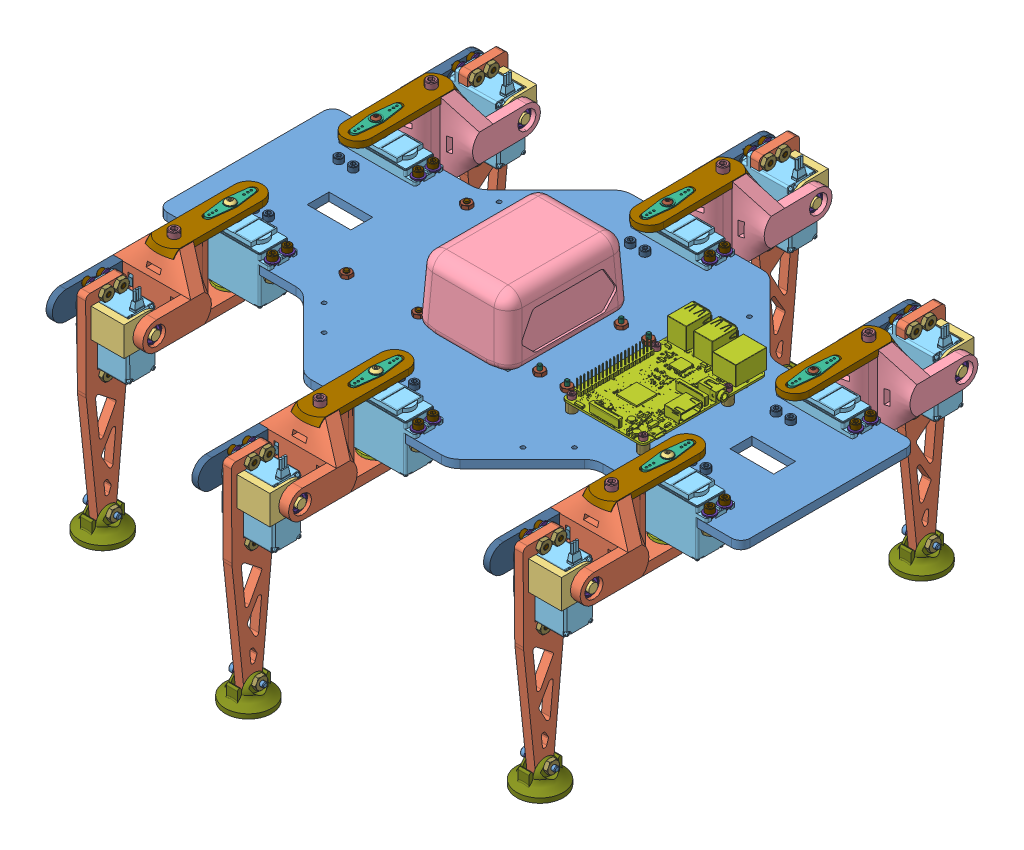
SolidWorks assembly Hexapod, configuration Défaut. Lengths in mm.
Overall size (400 185.52 400.77).
362 component instances, 31 part files, 135 mates.
Components (placement in the parent):
- Body-1: Body [Default] at (-400 -5.6 40) x (1 0 0) z (0 1 0) size (400 220 5.6)
- Leg_(Straight_Foot)-1: Leg_(Straight_Foot) [Default] at (-69.94 -26.67 -0.094) size (71.21 162.26 125.97) (flexible)
  - Foot_(Straight)-1: Foot_(Straight) [Default] at (4.9357 4.6704 -91.3697) x (0.014203 -0.004273 0.99989) z (-0.999899 0 0.014203) size (28 145.4 6)
  - bearing_mount_foot-1: bearing_mount_foot [Default] at (4.8169 16.6442 -99.7278) x (-0.014203 0.004273 -0.99989) z (0.999899 0 -0.014203) size (25 20 29.5)
  - Joint-1: Joint [Défaut] at (35.768 26.4662 -54.7315) x (-0.014203 0 -0.999899) z (0 1 0) size (96.52 53.26 53.26)
  - hs-422-2: hs-422 [Défaut] at (5.1023 6.612 -77.4562) x (-0.014203 0.004273 -0.99989) z (0.000061 0.999991 0.004272) size (19.81 42.09 58.23)
  - hs-422-3: hs-422 [Défaut] at (19.939 20.701 -19.812) x (0 0 1) z (-1 0 0) size (19.81 42.09 58.23)
  - hs-422_horn_straight-1: hs-422_horn_straight [Default] at (-16.9088 16.9412 -87.0065) x (0.014203 0 0.999899) z (0 1 0) size (33.93 4.93 8.79)
  - hs-422_horn_straight-2: hs-422_horn_straight [Default] at (9.652 42.5743 -9.906) x (-0.014203 0 -0.999899) z (-0.999899 0 0.014203) size (33.93 4.93 8.79)
  - Bearing_mount_leg-1: Bearing_mount_leg [Default] at (9.652 21 2.594) x (0 0 1) z (0 -1 0) size (35 20 30)
  - Bearing-1: Bearing [Default] at (9.652 -6.7498 -9.906) x (0.84763 0 0.530588) z (-0.530588 0 0.84763) size (13.87 4.75 13.87)
  - Bearing-2: Bearing [Default] at (32.2403 16.9412 -87.7047) x (0.007588 -0.845349 0.534161) z (-0.012007 -0.534214 -0.845264) size (13.87 4.75 13.87)
  - Joint_attachment_leg-1: Joint_attachment_leg [Défaut] at (35.768 26.4662 -54.7315) x (-0.014203 0 -0.999899) z (0 1 0) size (74.32 19.07 4.32)
  - Joint_attachment_foot-1: Joint_attachment_foot [Défaut] at (35.768 26.4662 -54.7315) x (-0.014203 0 -0.999899) z (0 1 0) size (64.08 6.7 19.07)
  - SBHCSCREW 0.112-40x0.25-HX-N-2: SBHCSCREW 0.112-40x0.25-HX-N [SBHCSCREW 0.112-40x0.25-HX-N] at (-19.9057 16.9412 -86.964) x (0.999899 0 -0.014203) z (-0.007102 0.866025 -0.49995) size (7.85 5.41 5.41)
  - SBHCSCREW 0.112-40x0.25-HX-N-3: SBHCSCREW 0.112-40x0.25-HX-N [SBHCSCREW 0.112-40x0.25-HX-N] at (9.652 45.5715 -9.906) x (0 -1 0) z (0.87304 0 0.487649) size (7.85 5.41 5.41)
  - MSHXNUT 0.138-32-D-N-15: MSHXNUT 0.138-32-D-N [MSHXNUT 0.138-32-D-N] at (5.0634 -17.1179 -82.3793) x (0.012331 0.496295 0.868066) z (-0.999899 0 0.014203) size (7.92 9.15 2.9)
  - MSHXNUT 0.138-32-D-N-16: MSHXNUT 0.138-32-D-N [MSHXNUT 0.138-32-D-N] at (4.9191 -17.0756 -92.5381) x (-0.01227 0.503696 -0.863794) z (-0.999899 0 0.014203) size (7.92 9.15 2.9)
  - MSHXNUT 0.138-32-D-N-17: MSHXNUT 0.138-32-D-N [MSHXNUT 0.138-32-D-N] at (5.0662 30.3817 -82.1827) x (0.000061 0.999991 0.004272) z (-0.999899 0 0.014203) size (7.92 9.15 2.9)
  - MSHXNUT 0.138-32-D-N-18: MSHXNUT 0.138-32-D-N [MSHXNUT 0.138-32-D-N] at (4.9219 30.4239 -92.3416) x (0.000061 0.999991 0.004272) z (-0.999899 0 0.014203) size (7.92 9.15 2.9)
  - HX-SHCS 0.164-32x0.5x0.5-N-1: HX-SHCS 0.164-32x0.5x0.5-N [HX-SHCS 0.164-32x0.5x0.5-N] at (9.1052 47.8568 -48.4) x (0 -1 0) z (0.014203 0 0.999899) size (16.87 6.86 6.86)
  - HX-SHCS 0.164-32x0.5x0.5-N-2: HX-SHCS 0.164-32x0.5x0.5-N [HX-SHCS 0.164-32x0.5x0.5-N] at (-21.967 16.9412 -59.205) x (0.999899 0 -0.014203) z (0.014203 0 0.999899) size (16.87 6.86 6.86)
  - MSHXNUT 0.164-32-D-N-11: MSHXNUT 0.164-32-D-N [MSHXNUT 0.164-32-D-N] at (9.1052 33.127 -48.4) x (0.87304 0 0.487649) z (0 1 0) size (8.74 10.09 3.3)
  - MSHXNUT 0.164-32-D-N-12: MSHXNUT 0.164-32-D-N [MSHXNUT 0.164-32-D-N] at (-7.2387 16.9412 -59.4142) x (0.014203 0 0.999899) z (-0.999899 0 0.014203) size (8.74 10.09 3.3)
  - HX-SHCS 0.112-40x0.5x0.5-N-7: HX-SHCS 0.112-40x0.5x0.5-N [HX-SHCS 0.112-40x0.5x0.5-N] at (-4.0273 11.7063 -99.6232) x (0.999899 0 -0.014203) z (0.014203 -0.004273 0.99989) size (15.54 4.65 4.65)
  - HX-SHCS 0.112-40x0.5x0.5-N-8: HX-SHCS 0.112-40x0.5x0.5-N [HX-SHCS 0.112-40x0.5x0.5-N] at (-4.0267 21.7062 -99.5805) x (0.999899 0 -0.014203) z (-0.014203 0.004273 -0.99989) size (15.54 4.65 4.65)
  - Slippers-1: Slippers [Default] at (1.9296 -111.2294 -91.7731) x (0.999899 0 -0.014203) z (0.014203 0 0.999899) size (35.48 18.25 37.71)
  - Narrow FW 0.138-1: Narrow FW 0.138 [Narrow FW 0.138] at (-3.4475 30.3814 -82.0597) x (0.999899 0 -0.014203) z (0.014203 0 0.999899) size (0.81 7.92 7.92)
  - HX-SHCS 0.138-32x0.5x0.5-N-2: HX-SHCS 0.138-32x0.5x0.5-N [HX-SHCS 0.138-32x0.5x0.5-N] at (-8.0191 30.3814 -81.9948) x (0.999899 0 -0.014203) z (0.014203 0 0.999899) size (16.21 5.74 5.74)
  - Narrow FW 0.138-2: Narrow FW 0.138 [Narrow FW 0.138] at (-3.4504 -17.1182 -82.2627) x (0.999899 0 -0.014203) z (0.014203 0 0.999899) size (0.81 7.92 7.92)
  - Narrow FW 0.138-3: Narrow FW 0.138 [Narrow FW 0.138] at (-3.5919 30.4248 -92.2186) x (0.999899 0 -0.014203) z (0.014203 0 0.999899) size (0.81 7.92 7.92)
  - Narrow FW 0.138-4: Narrow FW 0.138 [Narrow FW 0.138] at (-3.5947 -17.0748 -92.4216) x (0.999899 0 -0.014203) z (0.014203 0 0.999899) size (0.81 7.92 7.92)
  - HX-SHCS 0.138-32x0.5x0.5-N-3: HX-SHCS 0.138-32x0.5x0.5-N [HX-SHCS 0.138-32x0.5x0.5-N] at (-8.022 -17.1182 -82.1977) x (0.999899 0 -0.014203) z (0.014203 0 0.999899) size (16.21 5.74 5.74)
  - HX-SHCS 0.138-32x0.5x0.5-N-4: HX-SHCS 0.138-32x0.5x0.5-N [HX-SHCS 0.138-32x0.5x0.5-N] at (-8.1634 30.4248 -92.1537) x (0.999899 0 -0.014203) z (0.014203 0 0.999899) size (16.21 5.74 5.74)
  - HX-SHCS 0.138-32x0.5x0.5-N-5: HX-SHCS 0.138-32x0.5x0.5-N [HX-SHCS 0.138-32x0.5x0.5-N] at (-8.1663 -17.0748 -92.3566) x (0.999899 0 -0.014203) z (0.014203 0 0.999899) size (16.21 5.74 5.74)
  - HX-SHCS 0.138-32x0.5x0.5-N-6: HX-SHCS 0.138-32x0.5x0.5-N [HX-SHCS 0.138-32x0.5x0.5-N] at (-3.81 33.7566 -14.986) x (0 -1 0) z (-0.55878 0 0.829316) size (16.21 5.74 5.74)
  - Narrow FW 0.138-5: Narrow FW 0.138 [Narrow FW 0.138] at (-3.81 29.1846 -14.986) x (0 -1 0) z (0.55878 0 -0.829316) size (0.81 7.92 7.92)
  - Narrow FW 0.138-6: Narrow FW 0.138 [Narrow FW 0.138] at (43.69 29.1846 -14.986) x (0 -1 0) z (0.55878 0 -0.829316) size (0.81 7.92 7.92)
  - Narrow FW 0.138-7: Narrow FW 0.138 [Narrow FW 0.138] at (-3.81 29.1846 -4.826) x (0 -1 0) z (0.55878 0 -0.829316) size (0.81 7.92 7.92)
  - Narrow FW 0.138-8: Narrow FW 0.138 [Narrow FW 0.138] at (43.69 29.1846 -4.826) x (0 -1 0) z (0.55878 0 -0.829316) size (0.81 7.92 7.92)
  - HX-SHCS 0.138-32x0.5x0.5-N-7: HX-SHCS 0.138-32x0.5x0.5-N [HX-SHCS 0.138-32x0.5x0.5-N] at (43.69 33.7566 -14.986) x (0 -1 0) z (-0.55878 0 0.829316) size (16.21 5.74 5.74)
  - HX-SHCS 0.138-32x0.5x0.5-N-8: HX-SHCS 0.138-32x0.5x0.5-N [HX-SHCS 0.138-32x0.5x0.5-N] at (-3.81 33.7566 -4.826) x (0 -1 0) z (-0.55878 0 0.829316) size (16.21 5.74 5.74)
  - HX-SHCS 0.138-32x0.5x0.5-N-9: HX-SHCS 0.138-32x0.5x0.5-N [HX-SHCS 0.138-32x0.5x0.5-N] at (43.69 33.7566 -4.826) x (0 -1 0) z (-0.55878 0 0.829316) size (16.21 5.74 5.74)
  - HX-SHCS 0.138-32x0.75x0.75-N-10: HX-SHCS 0.138-32x0.75x0.75-N [HX-SHCS 0.138-32x0.75x0.75-N] at (-8.9913 -99.7294 -91.618) x (0.999899 0 -0.014203) z (-0.012539 -0.46966 -0.882758) size (22.56 5.74 5.74)
  - Narrow FW 0.138-10: Narrow FW 0.138 [Narrow FW 0.138] at (-5.2324 -99.7294 -91.6714) x (-0.999899 0 0.014203) z (-0.011665 -0.570502 -0.821213) size (0.81 7.92 7.92)
  - MSHXNUT 0.138-32-D-N-19: MSHXNUT 0.138-32-D-N [MSHXNUT 0.138-32-D-N] at (8.279 -99.7294 -91.8633) x (0 1 0) z (-0.999899 0 0.014203) size (7.92 9.15 2.9)
- Leg_(Straight_Foot)-2: Leg_(Straight_Foot) [Default] at (-369.94 -26.67 -0.094) size (71.21 162.26 125.97) (flexible)
  - Foot_(Straight)-1: Foot_(Straight) [Default] at (4.9357 4.6704 -91.3697) x (0.014203 -0.004273 0.99989) z (-0.999899 0 0.014203) size (28 145.4 6)
  - bearing_mount_foot-1: bearing_mount_foot [Default] at (4.8169 16.6442 -99.7278) x (-0.014203 0.004273 -0.99989) z (0.999899 0 -0.014203) size (25 20 29.5)
  - Joint-1: Joint [Défaut] at (35.768 26.4662 -54.7315) x (-0.014203 0 -0.999899) z (0 1 0) size (96.52 53.26 53.26)
  - hs-422-2: hs-422 [Défaut] at (5.1023 6.612 -77.4562) x (-0.014203 0.004273 -0.99989) z (0.000061 0.999991 0.004272) size (19.81 42.09 58.23)
  - hs-422-3: hs-422 [Défaut] at (19.939 20.701 -19.812) x (0 0 1) z (-1 0 0) size (19.81 42.09 58.23)
  - hs-422_horn_straight-1: hs-422_horn_straight [Default] at (-16.9088 16.9412 -87.0065) x (0.014203 0 0.999899) z (0 1 0) size (33.93 4.93 8.79)
  - hs-422_horn_straight-2: hs-422_horn_straight [Default] at (9.652 42.5743 -9.906) x (-0.014203 0 -0.999899) z (-0.999899 0 0.014203) size (33.93 4.93 8.79)
  - Bearing_mount_leg-1: Bearing_mount_leg [Default] at (9.652 21 2.594) x (0 0 1) z (0 -1 0) size (35 20 30)
  - Bearing-1: Bearing [Default] at (9.652 -6.7498 -9.906) x (0.84763 0 0.530588) z (-0.530588 0 0.84763) size (13.87 4.75 13.87)
  - Bearing-2: Bearing [Default] at (32.2403 16.9412 -87.7047) x (0.007588 -0.845349 0.534161) z (-0.012007 -0.534214 -0.845264) size (13.87 4.75 13.87)
  - Joint_attachment_leg-1: Joint_attachment_leg [Défaut] at (35.768 26.4662 -54.7315) x (-0.014203 0 -0.999899) z (0 1 0) size (74.32 19.07 4.32)
  - Joint_attachment_foot-1: Joint_attachment_foot [Défaut] at (35.768 26.4662 -54.7315) x (-0.014203 0 -0.999899) z (0 1 0) size (64.08 6.7 19.07)
  - SBHCSCREW 0.112-40x0.25-HX-N-2: SBHCSCREW 0.112-40x0.25-HX-N [SBHCSCREW 0.112-40x0.25-HX-N] at (-19.9057 16.9412 -86.964) x (0.999899 0 -0.014203) z (-0.007102 0.866025 -0.49995) size (7.85 5.41 5.41)
  - SBHCSCREW 0.112-40x0.25-HX-N-3: SBHCSCREW 0.112-40x0.25-HX-N [SBHCSCREW 0.112-40x0.25-HX-N] at (9.652 45.5715 -9.906) x (0 -1 0) z (0.87304 0 0.487649) size (7.85 5.41 5.41)
  - MSHXNUT 0.138-32-D-N-15: MSHXNUT 0.138-32-D-N [MSHXNUT 0.138-32-D-N] at (5.0634 -17.1179 -82.3793) x (0.012331 0.496295 0.868066) z (-0.999899 0 0.014203) size (7.92 9.15 2.9)
  - MSHXNUT 0.138-32-D-N-16: MSHXNUT 0.138-32-D-N [MSHXNUT 0.138-32-D-N] at (4.9191 -17.0756 -92.5381) x (-0.01227 0.503696 -0.863794) z (-0.999899 0 0.014203) size (7.92 9.15 2.9)
  - MSHXNUT 0.138-32-D-N-17: MSHXNUT 0.138-32-D-N [MSHXNUT 0.138-32-D-N] at (5.0662 30.3817 -82.1827) x (0.000061 0.999991 0.004272) z (-0.999899 0 0.014203) size (7.92 9.15 2.9)
  - MSHXNUT 0.138-32-D-N-18: MSHXNUT 0.138-32-D-N [MSHXNUT 0.138-32-D-N] at (4.9219 30.4239 -92.3416) x (0.000061 0.999991 0.004272) z (-0.999899 0 0.014203) size (7.92 9.15 2.9)
  - HX-SHCS 0.164-32x0.5x0.5-N-1: HX-SHCS 0.164-32x0.5x0.5-N [HX-SHCS 0.164-32x0.5x0.5-N] at (9.1052 47.8568 -48.4) x (0 -1 0) z (0.014203 0 0.999899) size (16.87 6.86 6.86)
  - HX-SHCS 0.164-32x0.5x0.5-N-2: HX-SHCS 0.164-32x0.5x0.5-N [HX-SHCS 0.164-32x0.5x0.5-N] at (-21.967 16.9412 -59.205) x (0.999899 0 -0.014203) z (0.014203 0 0.999899) size (16.87 6.86 6.86)
  - MSHXNUT 0.164-32-D-N-11: MSHXNUT 0.164-32-D-N [MSHXNUT 0.164-32-D-N] at (9.1052 33.127 -48.4) x (0.87304 0 0.487649) z (0 1 0) size (8.74 10.09 3.3)
  - MSHXNUT 0.164-32-D-N-12: MSHXNUT 0.164-32-D-N [MSHXNUT 0.164-32-D-N] at (-7.2387 16.9412 -59.4142) x (0.014203 0 0.999899) z (-0.999899 0 0.014203) size (8.74 10.09 3.3)
  - HX-SHCS 0.112-40x0.5x0.5-N-7: HX-SHCS 0.112-40x0.5x0.5-N [HX-SHCS 0.112-40x0.5x0.5-N] at (-4.0273 11.7063 -99.6232) x (0.999899 0 -0.014203) z (0.014203 -0.004273 0.99989) size (15.54 4.65 4.65)
  - HX-SHCS 0.112-40x0.5x0.5-N-8: HX-SHCS 0.112-40x0.5x0.5-N [HX-SHCS 0.112-40x0.5x0.5-N] at (-4.0267 21.7062 -99.5805) x (0.999899 0 -0.014203) z (-0.014203 0.004273 -0.99989) size (15.54 4.65 4.65)
  - Slippers-1: Slippers [Default] at (1.9296 -111.2294 -91.7731) x (0.999899 0 -0.014203) z (0.014203 0 0.999899) size (35.48 18.25 37.71)
  - Narrow FW 0.138-1: Narrow FW 0.138 [Narrow FW 0.138] at (-3.4475 30.3814 -82.0597) x (0.999899 0 -0.014203) z (0.014203 0 0.999899) size (0.81 7.92 7.92)
  - HX-SHCS 0.138-32x0.5x0.5-N-2: HX-SHCS 0.138-32x0.5x0.5-N [HX-SHCS 0.138-32x0.5x0.5-N] at (-8.0191 30.3814 -81.9948) x (0.999899 0 -0.014203) z (0.014203 0 0.999899) size (16.21 5.74 5.74)
  - Narrow FW 0.138-2: Narrow FW 0.138 [Narrow FW 0.138] at (-3.4504 -17.1182 -82.2627) x (0.999899 0 -0.014203) z (0.014203 0 0.999899) size (0.81 7.92 7.92)
  - Narrow FW 0.138-3: Narrow FW 0.138 [Narrow FW 0.138] at (-3.5919 30.4248 -92.2186) x (0.999899 0 -0.014203) z (0.014203 0 0.999899) size (0.81 7.92 7.92)
  - Narrow FW 0.138-4: Narrow FW 0.138 [Narrow FW 0.138] at (-3.5947 -17.0748 -92.4216) x (0.999899 0 -0.014203) z (0.014203 0 0.999899) size (0.81 7.92 7.92)
  - HX-SHCS 0.138-32x0.5x0.5-N-3: HX-SHCS 0.138-32x0.5x0.5-N [HX-SHCS 0.138-32x0.5x0.5-N] at (-8.022 -17.1182 -82.1977) x (0.999899 0 -0.014203) z (0.014203 0 0.999899) size (16.21 5.74 5.74)
  - HX-SHCS 0.138-32x0.5x0.5-N-4: HX-SHCS 0.138-32x0.5x0.5-N [HX-SHCS 0.138-32x0.5x0.5-N] at (-8.1634 30.4248 -92.1537) x (0.999899 0 -0.014203) z (0.014203 0 0.999899) size (16.21 5.74 5.74)
  - HX-SHCS 0.138-32x0.5x0.5-N-5: HX-SHCS 0.138-32x0.5x0.5-N [HX-SHCS 0.138-32x0.5x0.5-N] at (-8.1663 -17.0748 -92.3566) x (0.999899 0 -0.014203) z (0.014203 0 0.999899) size (16.21 5.74 5.74)
  - HX-SHCS 0.138-32x0.5x0.5-N-6: HX-SHCS 0.138-32x0.5x0.5-N [HX-SHCS 0.138-32x0.5x0.5-N] at (-3.81 33.7566 -14.986) x (0 -1 0) z (-0.55878 0 0.829316) size (16.21 5.74 5.74)
  - Narrow FW 0.138-5: Narrow FW 0.138 [Narrow FW 0.138] at (-3.81 29.1846 -14.986) x (0 -1 0) z (0.55878 0 -0.829316) size (0.81 7.92 7.92)
  - Narrow FW 0.138-6: Narrow FW 0.138 [Narrow FW 0.138] at (43.69 29.1846 -14.986) x (0 -1 0) z (0.55878 0 -0.829316) size (0.81 7.92 7.92)
  - Narrow FW 0.138-7: Narrow FW 0.138 [Narrow FW 0.138] at (-3.81 29.1846 -4.826) x (0 -1 0) z (0.55878 0 -0.829316) size (0.81 7.92 7.92)
  - Narrow FW 0.138-8: Narrow FW 0.138 [Narrow FW 0.138] at (43.69 29.1846 -4.826) x (0 -1 0) z (0.55878 0 -0.829316) size (0.81 7.92 7.92)
  - HX-SHCS 0.138-32x0.5x0.5-N-7: HX-SHCS 0.138-32x0.5x0.5-N [HX-SHCS 0.138-32x0.5x0.5-N] at (43.69 33.7566 -14.986) x (0 -1 0) z (-0.55878 0 0.829316) size (16.21 5.74 5.74)
  - HX-SHCS 0.138-32x0.5x0.5-N-8: HX-SHCS 0.138-32x0.5x0.5-N [HX-SHCS 0.138-32x0.5x0.5-N] at (-3.81 33.7566 -4.826) x (0 -1 0) z (-0.55878 0 0.829316) size (16.21 5.74 5.74)
  - HX-SHCS 0.138-32x0.5x0.5-N-9: HX-SHCS 0.138-32x0.5x0.5-N [HX-SHCS 0.138-32x0.5x0.5-N] at (43.69 33.7566 -4.826) x (0 -1 0) z (-0.55878 0 0.829316) size (16.21 5.74 5.74)
  - HX-SHCS 0.138-32x0.75x0.75-N-10: HX-SHCS 0.138-32x0.75x0.75-N [HX-SHCS 0.138-32x0.75x0.75-N] at (-8.9913 -99.7294 -91.618) x (0.999899 0 -0.014203) z (-0.012539 -0.46966 -0.882758) size (22.56 5.74 5.74)
  - Narrow FW 0.138-10: Narrow FW 0.138 [Narrow FW 0.138] at (-5.2324 -99.7294 -91.6714) x (-0.999899 0 0.014203) z (-0.011665 -0.570502 -0.821213) size (0.81 7.92 7.92)
  - MSHXNUT 0.138-32-D-N-19: MSHXNUT 0.138-32-D-N [MSHXNUT 0.138-32-D-N] at (8.279 -99.7294 -91.8633) x (0 1 0) z (-0.999899 0 0.014203) size (7.92 9.15 2.9)
- Leg_(Straight_Foot)-3: Leg_(Straight_Foot) [Default] at (-219.94 -26.67 -50.094) size (71.21 162.26 125.97) (flexible)
  - Foot_(Straight)-1: Foot_(Straight) [Default] at (4.9357 4.6704 -91.3697) x (0.014203 -0.004273 0.99989) z (-0.999899 0 0.014203) size (28 145.4 6)
  - bearing_mount_foot-1: bearing_mount_foot [Default] at (4.8169 16.6442 -99.7278) x (-0.014203 0.004273 -0.99989) z (0.999899 0 -0.014203) size (25 20 29.5)
  - Joint-1: Joint [Défaut] at (35.768 26.4662 -54.7315) x (-0.014203 0 -0.999899) z (0 1 0) size (96.52 53.26 53.26)
  - hs-422-2: hs-422 [Défaut] at (5.1023 6.612 -77.4562) x (-0.014203 0.004273 -0.99989) z (0.000061 0.999991 0.004272) size (19.81 42.09 58.23)
  - hs-422-3: hs-422 [Défaut] at (19.939 20.701 -19.812) x (0 0 1) z (-1 0 0) size (19.81 42.09 58.23)
  - hs-422_horn_straight-1: hs-422_horn_straight [Default] at (-16.9088 16.9412 -87.0065) x (0.014203 0 0.999899) z (0 1 0) size (33.93 4.93 8.79)
  - hs-422_horn_straight-2: hs-422_horn_straight [Default] at (9.652 42.5743 -9.906) x (-0.014203 0 -0.999899) z (-0.999899 0 0.014203) size (33.93 4.93 8.79)
  - Bearing_mount_leg-1: Bearing_mount_leg [Default] at (9.652 21 2.594) x (0 0 1) z (0 -1 0) size (35 20 30)
  - Bearing-1: Bearing [Default] at (9.652 -6.7498 -9.906) x (0.84763 0 0.530588) z (-0.530588 0 0.84763) size (13.87 4.75 13.87)
  - Bearing-2: Bearing [Default] at (32.2403 16.9412 -87.7047) x (0.007588 -0.845349 0.534161) z (-0.012007 -0.534214 -0.845264) size (13.87 4.75 13.87)
  - Joint_attachment_leg-1: Joint_attachment_leg [Défaut] at (35.768 26.4662 -54.7315) x (-0.014203 0 -0.999899) z (0 1 0) size (74.32 19.07 4.32)
  - Joint_attachment_foot-1: Joint_attachment_foot [Défaut] at (35.768 26.4662 -54.7315) x (-0.014203 0 -0.999899) z (0 1 0) size (64.08 6.7 19.07)
  - SBHCSCREW 0.112-40x0.25-HX-N-2: SBHCSCREW 0.112-40x0.25-HX-N [SBHCSCREW 0.112-40x0.25-HX-N] at (-19.9057 16.9412 -86.964) x (0.999899 0 -0.014203) z (-0.007102 0.866025 -0.49995) size (7.85 5.41 5.41)
  - SBHCSCREW 0.112-40x0.25-HX-N-3: SBHCSCREW 0.112-40x0.25-HX-N [SBHCSCREW 0.112-40x0.25-HX-N] at (9.652 45.5715 -9.906) x (0 -1 0) z (0.87304 0 0.487649) size (7.85 5.41 5.41)
  - MSHXNUT 0.138-32-D-N-15: MSHXNUT 0.138-32-D-N [MSHXNUT 0.138-32-D-N] at (5.0634 -17.1179 -82.3793) x (0.012331 0.496295 0.868066) z (-0.999899 0 0.014203) size (7.92 9.15 2.9)
  - MSHXNUT 0.138-32-D-N-16: MSHXNUT 0.138-32-D-N [MSHXNUT 0.138-32-D-N] at (4.9191 -17.0756 -92.5381) x (-0.01227 0.503696 -0.863794) z (-0.999899 0 0.014203) size (7.92 9.15 2.9)
  - MSHXNUT 0.138-32-D-N-17: MSHXNUT 0.138-32-D-N [MSHXNUT 0.138-32-D-N] at (5.0662 30.3817 -82.1827) x (0.000061 0.999991 0.004272) z (-0.999899 0 0.014203) size (7.92 9.15 2.9)
  - MSHXNUT 0.138-32-D-N-18: MSHXNUT 0.138-32-D-N [MSHXNUT 0.138-32-D-N] at (4.9219 30.4239 -92.3416) x (0.000061 0.999991 0.004272) z (-0.999899 0 0.014203) size (7.92 9.15 2.9)
  - HX-SHCS 0.164-32x0.5x0.5-N-1: HX-SHCS 0.164-32x0.5x0.5-N [HX-SHCS 0.164-32x0.5x0.5-N] at (9.1052 47.8568 -48.4) x (0 -1 0) z (0.014203 0 0.999899) size (16.87 6.86 6.86)
  - HX-SHCS 0.164-32x0.5x0.5-N-2: HX-SHCS 0.164-32x0.5x0.5-N [HX-SHCS 0.164-32x0.5x0.5-N] at (-21.967 16.9412 -59.205) x (0.999899 0 -0.014203) z (0.014203 0 0.999899) size (16.87 6.86 6.86)
  - MSHXNUT 0.164-32-D-N-11: MSHXNUT 0.164-32-D-N [MSHXNUT 0.164-32-D-N] at (9.1052 33.127 -48.4) x (0.87304 0 0.487649) z (0 1 0) size (8.74 10.09 3.3)
  - MSHXNUT 0.164-32-D-N-12: MSHXNUT 0.164-32-D-N [MSHXNUT 0.164-32-D-N] at (-7.2387 16.9412 -59.4142) x (0.014203 0 0.999899) z (-0.999899 0 0.014203) size (8.74 10.09 3.3)
  - HX-SHCS 0.112-40x0.5x0.5-N-7: HX-SHCS 0.112-40x0.5x0.5-N [HX-SHCS 0.112-40x0.5x0.5-N] at (-4.0273 11.7063 -99.6232) x (0.999899 0 -0.014203) z (0.014203 -0.004273 0.99989) size (15.54 4.65 4.65)
  - HX-SHCS 0.112-40x0.5x0.5-N-8: HX-SHCS 0.112-40x0.5x0.5-N [HX-SHCS 0.112-40x0.5x0.5-N] at (-4.0267 21.7062 -99.5805) x (0.999899 0 -0.014203) z (-0.014203 0.004273 -0.99989) size (15.54 4.65 4.65)
  - Slippers-1: Slippers [Default] at (1.9296 -111.2294 -91.7731) x (0.999899 0 -0.014203) z (0.014203 0 0.999899) size (35.48 18.25 37.71)
  - Narrow FW 0.138-1: Narrow FW 0.138 [Narrow FW 0.138] at (-3.4475 30.3814 -82.0597) x (0.999899 0 -0.014203) z (0.014203 0 0.999899) size (0.81 7.92 7.92)
  - HX-SHCS 0.138-32x0.5x0.5-N-2: HX-SHCS 0.138-32x0.5x0.5-N [HX-SHCS 0.138-32x0.5x0.5-N] at (-8.0191 30.3814 -81.9948) x (0.999899 0 -0.014203) z (0.014203 0 0.999899) size (16.21 5.74 5.74)
  - Narrow FW 0.138-2: Narrow FW 0.138 [Narrow FW 0.138] at (-3.4504 -17.1182 -82.2627) x (0.999899 0 -0.014203) z (0.014203 0 0.999899) size (0.81 7.92 7.92)
  - Narrow FW 0.138-3: Narrow FW 0.138 [Narrow FW 0.138] at (-3.5919 30.4248 -92.2186) x (0.999899 0 -0.014203) z (0.014203 0 0.999899) size (0.81 7.92 7.92)
  - Narrow FW 0.138-4: Narrow FW 0.138 [Narrow FW 0.138] at (-3.5947 -17.0748 -92.4216) x (0.999899 0 -0.014203) z (0.014203 0 0.999899) size (0.81 7.92 7.92)
  - HX-SHCS 0.138-32x0.5x0.5-N-3: HX-SHCS 0.138-32x0.5x0.5-N [HX-SHCS 0.138-32x0.5x0.5-N] at (-8.022 -17.1182 -82.1977) x (0.999899 0 -0.014203) z (0.014203 0 0.999899) size (16.21 5.74 5.74)
  - HX-SHCS 0.138-32x0.5x0.5-N-4: HX-SHCS 0.138-32x0.5x0.5-N [HX-SHCS 0.138-32x0.5x0.5-N] at (-8.1634 30.4248 -92.1537) x (0.999899 0 -0.014203) z (0.014203 0 0.999899) size (16.21 5.74 5.74)
  - HX-SHCS 0.138-32x0.5x0.5-N-5: HX-SHCS 0.138-32x0.5x0.5-N [HX-SHCS 0.138-32x0.5x0.5-N] at (-8.1663 -17.0748 -92.3566) x (0.999899 0 -0.014203) z (0.014203 0 0.999899) size (16.21 5.74 5.74)
  - HX-SHCS 0.138-32x0.5x0.5-N-6: HX-SHCS 0.138-32x0.5x0.5-N [HX-SHCS 0.138-32x0.5x0.5-N] at (-3.81 33.7566 -14.986) x (0 -1 0) z (-0.55878 0 0.829316) size (16.21 5.74 5.74)
  - Narrow FW 0.138-5: Narrow FW 0.138 [Narrow FW 0.138] at (-3.81 29.1846 -14.986) x (0 -1 0) z (0.55878 0 -0.829316) size (0.81 7.92 7.92)
  - Narrow FW 0.138-6: Narrow FW 0.138 [Narrow FW 0.138] at (43.69 29.1846 -14.986) x (0 -1 0) z (0.55878 0 -0.829316) size (0.81 7.92 7.92)
  - Narrow FW 0.138-7: Narrow FW 0.138 [Narrow FW 0.138] at (-3.81 29.1846 -4.826) x (0 -1 0) z (0.55878 0 -0.829316) size (0.81 7.92 7.92)
  - Narrow FW 0.138-8: Narrow FW 0.138 [Narrow FW 0.138] at (43.69 29.1846 -4.826) x (0 -1 0) z (0.55878 0 -0.829316) size (0.81 7.92 7.92)
  - HX-SHCS 0.138-32x0.5x0.5-N-7: HX-SHCS 0.138-32x0.5x0.5-N [HX-SHCS 0.138-32x0.5x0.5-N] at (43.69 33.7566 -14.986) x (0 -1 0) z (-0.55878 0 0.829316) size (16.21 5.74 5.74)
  - HX-SHCS 0.138-32x0.5x0.5-N-8: HX-SHCS 0.138-32x0.5x0.5-N [HX-SHCS 0.138-32x0.5x0.5-N] at (-3.81 33.7566 -4.826) x (0 -1 0) z (-0.55878 0 0.829316) size (16.21 5.74 5.74)
  - HX-SHCS 0.138-32x0.5x0.5-N-9: HX-SHCS 0.138-32x0.5x0.5-N [HX-SHCS 0.138-32x0.5x0.5-N] at (43.69 33.7566 -4.826) x (0 -1 0) z (-0.55878 0 0.829316) size (16.21 5.74 5.74)
  - HX-SHCS 0.138-32x0.75x0.75-N-10: HX-SHCS 0.138-32x0.75x0.75-N [HX-SHCS 0.138-32x0.75x0.75-N] at (-8.9913 -99.7294 -91.618) x (0.999899 0 -0.014203) z (-0.012539 -0.46966 -0.882758) size (22.56 5.74 5.74)
  - Narrow FW 0.138-10: Narrow FW 0.138 [Narrow FW 0.138] at (-5.2324 -99.7294 -91.6714) x (-0.999899 0 0.014203) z (-0.011665 -0.570502 -0.821213) size (0.81 7.92 7.92)
  - MSHXNUT 0.138-32-D-N-19: MSHXNUT 0.138-32-D-N [MSHXNUT 0.138-32-D-N] at (8.279 -99.7294 -91.8633) x (0 1 0) z (-0.999899 0 0.014203) size (7.92 9.15 2.9)
- Leg_(Straight_Foot)_(Mirror)-1: Leg_(Straight_Foot)_(Mirror) [Default] at (-369.94 -26.67 99.906) size (70.36 162.3 124.8) (flexible)
  - Joint_(Mirror)-1: Joint_(Mirror) [Défaut] at (36.4933 -51.1276 34.4889) x (0.002055 0 0.999998) z (0 -1 0) size (96.52 53.26 53.26)
  - hs-422-3: hs-422 [Défaut] at (19.939 20.701 -19.812) x (0 0 1) z (-1 0 0) size (19.81 42.09 58.23)
  - hs-422_horn_straight-2: hs-422_horn_straight [Default] at (9.652 42.5743 -9.906) x (0.002055 0 0.999998) z (0.999998 0 -0.002055) size (33.93 4.93 8.79)
  - Bearing_mount_leg-1: Bearing_mount_leg [Default] at (9.652 21 -22.406) x (0 0 -1) z (0 -1 0) size (35 20 30)
  - Bearing-1: Bearing [Default] at (9.652 -6.7498 -9.906) x (0.266287 0 0.963894) z (-0.963894 0 0.266287) size (13.87 4.75 13.87)
  - Joint_attachment_leg-1: Joint_attachment_leg [Défaut] at (-17.0066 26.5024 34.5989) x (0.002055 0 0.999998) z (0 1 0) size (74.32 19.07 4.32)
  - bearing_mount_foot-2: bearing_mount_foot [Default] at (6.7141 17.2663 79.9818) x (0.002055 -0.004919 0.999986) z (0.999998 0 -0.002055) size (25 20 29.5)
  - Bearing-3: Bearing [Default] at (29.1886 16.9774 67.524) x (-0.001098 -0.845349 -0.534213) z (0.001738 -0.534214 0.845347) size (13.87 4.75 13.87)
  - hs-422-4: hs-422 [Défaut] at (6.0779 6.6418 77.4268) x (-0.002055 0.004919 -0.999986) z (0.00001 0.999988 0.004919) size (19.81 42.09 58.23)
  - hs-422_horn_straight-3: hs-422_horn_straight [Default] at (-15.8156 16.9774 67.6165) x (-0.002055 0 -0.999998) z (0 -1 0) size (33.93 4.93 8.79)
  - Foot_(Straight)-2: Foot_(Straight) [Default] at (0.0967 4.6719 71.5233) x (-0.002055 0.004919 -0.999986) z (0.999998 0 -0.002055) size (28 145.4 6)
  - Joint_attachment_foot-2: Joint_attachment_foot [Défaut] at (36.4933 7.4524 34.4889) x (0.002055 0 0.999998) z (0 -1 0) size (64.08 6.7 19.07)
  - SBHCSCREW 0.138-32x0.25-HX-N-1: SBHCSCREW 0.138-32x0.25-HX-N [SBHCSCREW 0.138-32x0.25-HX-N] at (-19.1684 16.9774 67.6234) x (0.999998 0 -0.002055) z (0.002055 0 0.999998) size (8.2 6.65 6.65)
  - SBHCSCREW 0.138-32x0.25-HX-N-2: SBHCSCREW 0.138-32x0.25-HX-N [SBHCSCREW 0.138-32x0.25-HX-N] at (9.652 45.9271 -9.906) x (0 -1 0) z (-0.864996 0 0.501779) size (8.2 6.65 6.65)
  - HX-SHCS 0.112-40x0.5x0.5-N-5: HX-SHCS 0.112-40x0.5x0.5-N [HX-SHCS 0.112-40x0.5x0.5-N] at (-2.7306 21.6303 80.0227) x (0.999998 0 -0.002055) z (0.001019 -0.868474 0.495733) size (15.54 4.65 4.65)
  - HX-SHCS 0.112-40x0.5x0.5-N-6: HX-SHCS 0.112-40x0.5x0.5-N [HX-SHCS 0.112-40x0.5x0.5-N] at (-2.7307 11.6304 79.9735) x (0.999998 0 -0.002055) z (0.001036 0.863555 0.504253) size (15.54 4.65 4.65)
  - HX-SHCS 0.164-32x0.5x0.5-N-3: HX-SHCS 0.164-32x0.5x0.5-N [HX-SHCS 0.164-32x0.5x0.5-N] at (-21.1613 16.9774 39.9006) x (0.999998 0 -0.002055) z (0.001028 0.866025 0.499999) size (16.87 6.86 6.86)
  - HX-SHCS 0.164-32x0.5x0.5-N-4: HX-SHCS 0.164-32x0.5x0.5-N [HX-SHCS 0.164-32x0.5x0.5-N] at (9.7311 47.893 28.5918) x (0 -1 0) z (0.002055 0 0.999998) size (16.87 6.86 6.86)
  - MSHXNUT 0.138-32-D-N-14: MSHXNUT 0.138-32-D-N [MSHXNUT 0.138-32-D-N] at (6.0779 -17.0332 62.3241) x (-0.001785 -0.495734 -0.868473) z (-0.999998 0 0.002055) size (7.92 9.15 2.9)
  - MSHXNUT 0.138-32-D-N-15: MSHXNUT 0.138-32-D-N [MSHXNUT 0.138-32-D-N] at (8.9943 -17.0832 72.478) x (-0.001775 0.504254 -0.863554) z (0.999998 0 -0.002055) size (7.92 9.15 2.9)
  - MSHXNUT 0.138-32-D-N-16: MSHXNUT 0.138-32-D-N [MSHXNUT 0.138-32-D-N] at (8.9739 30.4662 62.5518) x (0.00001 0.999988 0.004919) z (0.999998 0 -0.002055) size (7.92 9.15 2.9)
  - MSHXNUT 0.138-32-D-N-17: MSHXNUT 0.138-32-D-N [MSHXNUT 0.138-32-D-N] at (6.0992 30.4162 72.7176) x (-0.001785 -0.495734 -0.868473) z (-0.999998 0 0.002055) size (7.92 9.15 2.9)
  - MSHXNUT 0.164-32-D-N-10: MSHXNUT 0.164-32-D-N [MSHXNUT 0.164-32-D-N] at (-6.4315 16.9774 39.8703) x (0.002055 0 0.999998) z (-0.999998 0 0.002055) size (8.74 10.09 3.3)
  - MSHXNUT 0.164-32-D-N-11: MSHXNUT 0.164-32-D-N [MSHXNUT 0.164-32-D-N] at (9.7311 29.8612 28.5918) x (-0.002055 0 -0.999998) z (0 -1 0) size (8.74 10.09 3.3)
  - Slippers-1: Slippers [Default] at (3.0957 -111.2276 71.0036) x (0.999998 0 -0.002055) z (0.002055 0 0.999998) size (35.48 18.25 37.71)
  - Narrow FW 0.138-4: Narrow FW 0.138 [Narrow FW 0.138] at (-2.4363 30.4642 62.5753) x (0.999998 0 -0.002055) z (0.002055 0 0.999998) size (0.81 7.92 7.92)
  - HX-SHCS 0.138-32x0.5x0.5-N-14: HX-SHCS 0.138-32x0.5x0.5-N [HX-SHCS 0.138-32x0.5x0.5-N] at (-7.0082 30.4642 62.5847) x (0.999998 0 -0.002055) z (0.002055 0 0.999998) size (16.21 5.74 5.74)
  - Narrow FW 0.138-5: Narrow FW 0.138 [Narrow FW 0.138] at (-2.4367 -17.0352 62.3416) x (0.999998 0 -0.002055) z (0.002055 0 0.999998) size (0.81 7.92 7.92)
  - Narrow FW 0.138-6: Narrow FW 0.138 [Narrow FW 0.138] at (-2.4154 30.4142 72.7351) x (0.999998 0 -0.002055) z (0.002055 0 0.999998) size (0.81 7.92 7.92)
  - Narrow FW 0.138-7: Narrow FW 0.138 [Narrow FW 0.138] at (-2.4158 -17.0852 72.5015) x (0.999998 0 -0.002055) z (0.002055 0 0.999998) size (0.81 7.92 7.92)
  - HX-SHCS 0.138-32x0.5x0.5-N-15: HX-SHCS 0.138-32x0.5x0.5-N [HX-SHCS 0.138-32x0.5x0.5-N] at (-7.0087 -17.0352 62.351) x (0.999998 0 -0.002055) z (0.002055 0 0.999998) size (16.21 5.74 5.74)
  - HX-SHCS 0.138-32x0.5x0.5-N-16: HX-SHCS 0.138-32x0.5x0.5-N [HX-SHCS 0.138-32x0.5x0.5-N] at (-6.9874 30.4142 72.7445) x (0.999998 0 -0.002055) z (0.002055 0 0.999998) size (16.21 5.74 5.74)
  - HX-SHCS 0.138-32x0.5x0.5-N-17: HX-SHCS 0.138-32x0.5x0.5-N [HX-SHCS 0.138-32x0.5x0.5-N] at (-6.9878 -17.0852 72.5109) x (0.999998 0 -0.002055) z (0.002055 0 0.999998) size (16.21 5.74 5.74)
  - Narrow FW 0.138-8: Narrow FW 0.138 [Narrow FW 0.138] at (-3.81 29.1846 -4.826) x (0 -1 0) z (0.55878 0 -0.829316) size (0.81 7.92 7.92)
  - HX-SHCS 0.138-32x0.5x0.5-N-18: HX-SHCS 0.138-32x0.5x0.5-N [HX-SHCS 0.138-32x0.5x0.5-N] at (-3.81 33.7566 -4.826) x (0 -1 0) z (-0.55878 0 0.829316) size (16.21 5.74 5.74)
  - Narrow FW 0.138-9: Narrow FW 0.138 [Narrow FW 0.138] at (43.69 29.1846 -4.826) x (0 -1 0) z (0.55878 0 -0.829316) size (0.81 7.92 7.92)
  - Narrow FW 0.138-10: Narrow FW 0.138 [Narrow FW 0.138] at (-3.81 29.1846 -14.986) x (0 -1 0) z (0.55878 0 -0.829316) size (0.81 7.92 7.92)
  - Narrow FW 0.138-11: Narrow FW 0.138 [Narrow FW 0.138] at (43.69 29.1846 -14.986) x (0 -1 0) z (0.55878 0 -0.829316) size (0.81 7.92 7.92)
  - HX-SHCS 0.138-32x0.5x0.5-N-19: HX-SHCS 0.138-32x0.5x0.5-N [HX-SHCS 0.138-32x0.5x0.5-N] at (43.69 33.7566 -4.826) x (0 -1 0) z (-0.55878 0 0.829316) size (16.21 5.74 5.74)
  - HX-SHCS 0.138-32x0.5x0.5-N-20: HX-SHCS 0.138-32x0.5x0.5-N [HX-SHCS 0.138-32x0.5x0.5-N] at (-3.81 33.7566 -14.986) x (0 -1 0) z (-0.55878 0 0.829316) size (16.21 5.74 5.74)
  - HX-SHCS 0.138-32x0.5x0.5-N-21: HX-SHCS 0.138-32x0.5x0.5-N [HX-SHCS 0.138-32x0.5x0.5-N] at (43.69 33.7566 -14.986) x (0 -1 0) z (-0.55878 0 0.829316) size (16.21 5.74 5.74)
  - HX-SHCS 0.138-32x0.75x0.75-N-1: HX-SHCS 0.138-32x0.75x0.75-N [HX-SHCS 0.138-32x0.75x0.75-N] at (-7.8263 -99.7276 71.0261) x (0.999998 0 -0.002055) z (-0.001815 -0.46966 -0.882845) size (22.56 5.74 5.74)
  - Narrow FW 0.138-12: Narrow FW 0.138 [Narrow FW 0.138] at (-4.0671 -99.7276 71.0183) x (-0.999998 0 0.002055) z (-0.001688 -0.570502 -0.821294) size (0.81 7.92 7.92)
  - MSHXNUT 0.138-32-D-N-18: MSHXNUT 0.138-32-D-N [MSHXNUT 0.138-32-D-N] at (9.4457 -99.7276 70.9906) x (0 1 0) z (-0.999998 0 0.002055) size (7.92 9.15 2.9)
- Leg_(Straight_Foot)_(Mirror)-2: Leg_(Straight_Foot)_(Mirror) [Default] at (-69.94 -26.67 99.906) size (70.36 162.3 124.8) (flexible)
  - Joint_(Mirror)-1: Joint_(Mirror) [Défaut] at (36.4933 -51.1276 34.4889) x (0.002055 0 0.999998) z (0 -1 0) size (96.52 53.26 53.26)
  - hs-422-3: hs-422 [Défaut] at (19.939 20.701 -19.812) x (0 0 1) z (-1 0 0) size (19.81 42.09 58.23)
  - hs-422_horn_straight-2: hs-422_horn_straight [Default] at (9.652 42.5743 -9.906) x (0.002055 0 0.999998) z (0.999998 0 -0.002055) size (33.93 4.93 8.79)
  - Bearing_mount_leg-1: Bearing_mount_leg [Default] at (9.652 21 -22.406) x (0 0 -1) z (0 -1 0) size (35 20 30)
  - Bearing-1: Bearing [Default] at (9.652 -6.7498 -9.906) x (0.266287 0 0.963894) z (-0.963894 0 0.266287) size (13.87 4.75 13.87)
  - Joint_attachment_leg-1: Joint_attachment_leg [Défaut] at (-17.0066 26.5024 34.5989) x (0.002055 0 0.999998) z (0 1 0) size (74.32 19.07 4.32)
  - bearing_mount_foot-2: bearing_mount_foot [Default] at (6.7141 17.2663 79.9818) x (0.002055 -0.004919 0.999986) z (0.999998 0 -0.002055) size (25 20 29.5)
  - Bearing-3: Bearing [Default] at (29.1886 16.9774 67.524) x (-0.001098 -0.845349 -0.534213) z (0.001738 -0.534214 0.845347) size (13.87 4.75 13.87)
  - hs-422-4: hs-422 [Défaut] at (6.0779 6.6418 77.4268) x (-0.002055 0.004919 -0.999986) z (0.00001 0.999988 0.004919) size (19.81 42.09 58.23)
  - hs-422_horn_straight-3: hs-422_horn_straight [Default] at (-15.8156 16.9774 67.6165) x (-0.002055 0 -0.999998) z (0 -1 0) size (33.93 4.93 8.79)
  - Foot_(Straight)-2: Foot_(Straight) [Default] at (0.0967 4.6719 71.5233) x (-0.002055 0.004919 -0.999986) z (0.999998 0 -0.002055) size (28 145.4 6)
  - Joint_attachment_foot-2: Joint_attachment_foot [Défaut] at (36.4933 7.4524 34.4889) x (0.002055 0 0.999998) z (0 -1 0) size (64.08 6.7 19.07)
  - SBHCSCREW 0.138-32x0.25-HX-N-1: SBHCSCREW 0.138-32x0.25-HX-N [SBHCSCREW 0.138-32x0.25-HX-N] at (-19.1684 16.9774 67.6234) x (0.999998 0 -0.002055) z (0.002055 0 0.999998) size (8.2 6.65 6.65)
  - SBHCSCREW 0.138-32x0.25-HX-N-2: SBHCSCREW 0.138-32x0.25-HX-N [SBHCSCREW 0.138-32x0.25-HX-N] at (9.652 45.9271 -9.906) x (0 -1 0) z (-0.864996 0 0.501779) size (8.2 6.65 6.65)
  - HX-SHCS 0.112-40x0.5x0.5-N-5: HX-SHCS 0.112-40x0.5x0.5-N [HX-SHCS 0.112-40x0.5x0.5-N] at (-2.7306 21.6303 80.0227) x (0.999998 0 -0.002055) z (0.001019 -0.868474 0.495733) size (15.54 4.65 4.65)
  - HX-SHCS 0.112-40x0.5x0.5-N-6: HX-SHCS 0.112-40x0.5x0.5-N [HX-SHCS 0.112-40x0.5x0.5-N] at (-2.7307 11.6304 79.9735) x (0.999998 0 -0.002055) z (0.001036 0.863555 0.504253) size (15.54 4.65 4.65)
  - HX-SHCS 0.164-32x0.5x0.5-N-3: HX-SHCS 0.164-32x0.5x0.5-N [HX-SHCS 0.164-32x0.5x0.5-N] at (-21.1613 16.9774 39.9006) x (0.999998 0 -0.002055) z (0.001028 0.866025 0.499999) size (16.87 6.86 6.86)
  - HX-SHCS 0.164-32x0.5x0.5-N-4: HX-SHCS 0.164-32x0.5x0.5-N [HX-SHCS 0.164-32x0.5x0.5-N] at (9.7311 47.893 28.5918) x (0 -1 0) z (0.002055 0 0.999998) size (16.87 6.86 6.86)
  - MSHXNUT 0.138-32-D-N-14: MSHXNUT 0.138-32-D-N [MSHXNUT 0.138-32-D-N] at (6.0779 -17.0332 62.3241) x (-0.001785 -0.495734 -0.868473) z (-0.999998 0 0.002055) size (7.92 9.15 2.9)
  - MSHXNUT 0.138-32-D-N-15: MSHXNUT 0.138-32-D-N [MSHXNUT 0.138-32-D-N] at (8.9943 -17.0832 72.478) x (-0.001775 0.504254 -0.863554) z (0.999998 0 -0.002055) size (7.92 9.15 2.9)
  - MSHXNUT 0.138-32-D-N-16: MSHXNUT 0.138-32-D-N [MSHXNUT 0.138-32-D-N] at (8.9739 30.4662 62.5518) x (0.00001 0.999988 0.004919) z (0.999998 0 -0.002055) size (7.92 9.15 2.9)
  - MSHXNUT 0.138-32-D-N-17: MSHXNUT 0.138-32-D-N [MSHXNUT 0.138-32-D-N] at (6.0992 30.4162 72.7176) x (-0.001785 -0.495734 -0.868473) z (-0.999998 0 0.002055) size (7.92 9.15 2.9)
  - MSHXNUT 0.164-32-D-N-10: MSHXNUT 0.164-32-D-N [MSHXNUT 0.164-32-D-N] at (-6.4315 16.9774 39.8703) x (0.002055 0 0.999998) z (-0.999998 0 0.002055) size (8.74 10.09 3.3)
  - MSHXNUT 0.164-32-D-N-11: MSHXNUT 0.164-32-D-N [MSHXNUT 0.164-32-D-N] at (9.7311 29.8612 28.5918) x (-0.002055 0 -0.999998) z (0 -1 0) size (8.74 10.09 3.3)
  - Slippers-1: Slippers [Default] at (3.0957 -111.2276 71.0036) x (0.999998 0 -0.002055) z (0.002055 0 0.999998) size (35.48 18.25 37.71)
  - Narrow FW 0.138-4: Narrow FW 0.138 [Narrow FW 0.138] at (-2.4363 30.4642 62.5753) x (0.999998 0 -0.002055) z (0.002055 0 0.999998) size (0.81 7.92 7.92)
  - HX-SHCS 0.138-32x0.5x0.5-N-14: HX-SHCS 0.138-32x0.5x0.5-N [HX-SHCS 0.138-32x0.5x0.5-N] at (-7.0082 30.4642 62.5847) x (0.999998 0 -0.002055) z (0.002055 0 0.999998) size (16.21 5.74 5.74)
  - Narrow FW 0.138-5: Narrow FW 0.138 [Narrow FW 0.138] at (-2.4367 -17.0352 62.3416) x (0.999998 0 -0.002055) z (0.002055 0 0.999998) size (0.81 7.92 7.92)
  - Narrow FW 0.138-6: Narrow FW 0.138 [Narrow FW 0.138] at (-2.4154 30.4142 72.7351) x (0.999998 0 -0.002055) z (0.002055 0 0.999998) size (0.81 7.92 7.92)
  - Narrow FW 0.138-7: Narrow FW 0.138 [Narrow FW 0.138] at (-2.4158 -17.0852 72.5015) x (0.999998 0 -0.002055) z (0.002055 0 0.999998) size (0.81 7.92 7.92)
  - HX-SHCS 0.138-32x0.5x0.5-N-15: HX-SHCS 0.138-32x0.5x0.5-N [HX-SHCS 0.138-32x0.5x0.5-N] at (-7.0087 -17.0352 62.351) x (0.999998 0 -0.002055) z (0.002055 0 0.999998) size (16.21 5.74 5.74)
  - HX-SHCS 0.138-32x0.5x0.5-N-16: HX-SHCS 0.138-32x0.5x0.5-N [HX-SHCS 0.138-32x0.5x0.5-N] at (-6.9874 30.4142 72.7445) x (0.999998 0 -0.002055) z (0.002055 0 0.999998) size (16.21 5.74 5.74)
  - HX-SHCS 0.138-32x0.5x0.5-N-17: HX-SHCS 0.138-32x0.5x0.5-N [HX-SHCS 0.138-32x0.5x0.5-N] at (-6.9878 -17.0852 72.5109) x (0.999998 0 -0.002055) z (0.002055 0 0.999998) size (16.21 5.74 5.74)
  - Narrow FW 0.138-8: Narrow FW 0.138 [Narrow FW 0.138] at (-3.81 29.1846 -4.826) x (0 -1 0) z (0.55878 0 -0.829316) size (0.81 7.92 7.92)
  - HX-SHCS 0.138-32x0.5x0.5-N-18: HX-SHCS 0.138-32x0.5x0.5-N [HX-SHCS 0.138-32x0.5x0.5-N] at (-3.81 33.7566 -4.826) x (0 -1 0) z (-0.55878 0 0.829316) size (16.21 5.74 5.74)
  - Narrow FW 0.138-9: Narrow FW 0.138 [Narrow FW 0.138] at (43.69 29.1846 -4.826) x (0 -1 0) z (0.55878 0 -0.829316) size (0.81 7.92 7.92)
  - Narrow FW 0.138-10: Narrow FW 0.138 [Narrow FW 0.138] at (-3.81 29.1846 -14.986) x (0 -1 0) z (0.55878 0 -0.829316) size (0.81 7.92 7.92)
  - Narrow FW 0.138-11: Narrow FW 0.138 [Narrow FW 0.138] at (43.69 29.1846 -14.986) x (0 -1 0) z (0.55878 0 -0.829316) size (0.81 7.92 7.92)
  - HX-SHCS 0.138-32x0.5x0.5-N-19: HX-SHCS 0.138-32x0.5x0.5-N [HX-SHCS 0.138-32x0.5x0.5-N] at (43.69 33.7566 -4.826) x (0 -1 0) z (-0.55878 0 0.829316) size (16.21 5.74 5.74)
  - HX-SHCS 0.138-32x0.5x0.5-N-20: HX-SHCS 0.138-32x0.5x0.5-N [HX-SHCS 0.138-32x0.5x0.5-N] at (-3.81 33.7566 -14.986) x (0 -1 0) z (-0.55878 0 0.829316) size (16.21 5.74 5.74)
  - HX-SHCS 0.138-32x0.5x0.5-N-21: HX-SHCS 0.138-32x0.5x0.5-N [HX-SHCS 0.138-32x0.5x0.5-N] at (43.69 33.7566 -14.986) x (0 -1 0) z (-0.55878 0 0.829316) size (16.21 5.74 5.74)
  - HX-SHCS 0.138-32x0.75x0.75-N-1: HX-SHCS 0.138-32x0.75x0.75-N [HX-SHCS 0.138-32x0.75x0.75-N] at (-7.8263 -99.7276 71.0261) x (0.999998 0 -0.002055) z (-0.001815 -0.46966 -0.882845) size (22.56 5.74 5.74)
  - Narrow FW 0.138-12: Narrow FW 0.138 [Narrow FW 0.138] at (-4.0671 -99.7276 71.0183) x (-0.999998 0 0.002055) z (-0.001688 -0.570502 -0.821294) size (0.81 7.92 7.92)
  - MSHXNUT 0.138-32-D-N-18: MSHXNUT 0.138-32-D-N [MSHXNUT 0.138-32-D-N] at (9.4457 -99.7276 70.9906) x (0 1 0) z (-0.999998 0 0.002055) size (7.92 9.15 2.9)
- Leg_(Straight_Foot)_(Mirror)-3: Leg_(Straight_Foot)_(Mirror) [Default] at (-219.94 -26.67 149.906) size (70.36 162.3 124.8) (flexible)
  - Joint_(Mirror)-1: Joint_(Mirror) [Défaut] at (36.4933 -51.1276 34.4889) x (0.002055 0 0.999998) z (0 -1 0) size (96.52 53.26 53.26)
  - hs-422-3: hs-422 [Défaut] at (19.939 20.701 -19.812) x (0 0 1) z (-1 0 0) size (19.81 42.09 58.23)
  - hs-422_horn_straight-2: hs-422_horn_straight [Default] at (9.652 42.5743 -9.906) x (0.002055 0 0.999998) z (0.999998 0 -0.002055) size (33.93 4.93 8.79)
  - Bearing_mount_leg-1: Bearing_mount_leg [Default] at (9.652 21 -22.406) x (0 0 -1) z (0 -1 0) size (35 20 30)
  - Bearing-1: Bearing [Default] at (9.652 -6.7498 -9.906) x (0.266287 0 0.963894) z (-0.963894 0 0.266287) size (13.87 4.75 13.87)
  - Joint_attachment_leg-1: Joint_attachment_leg [Défaut] at (-17.0066 26.5024 34.5989) x (0.002055 0 0.999998) z (0 1 0) size (74.32 19.07 4.32)
  - bearing_mount_foot-2: bearing_mount_foot [Default] at (6.7141 17.2663 79.9818) x (0.002055 -0.004919 0.999986) z (0.999998 0 -0.002055) size (25 20 29.5)
  - Bearing-3: Bearing [Default] at (29.1886 16.9774 67.524) x (-0.001098 -0.845349 -0.534213) z (0.001738 -0.534214 0.845347) size (13.87 4.75 13.87)
  - hs-422-4: hs-422 [Défaut] at (6.0779 6.6418 77.4268) x (-0.002055 0.004919 -0.999986) z (0.00001 0.999988 0.004919) size (19.81 42.09 58.23)
  - hs-422_horn_straight-3: hs-422_horn_straight [Default] at (-15.8156 16.9774 67.6165) x (-0.002055 0 -0.999998) z (0 -1 0) size (33.93 4.93 8.79)
  - Foot_(Straight)-2: Foot_(Straight) [Default] at (0.0967 4.6719 71.5233) x (-0.002055 0.004919 -0.999986) z (0.999998 0 -0.002055) size (28 145.4 6)
  - Joint_attachment_foot-2: Joint_attachment_foot [Défaut] at (36.4933 7.4524 34.4889) x (0.002055 0 0.999998) z (0 -1 0) size (64.08 6.7 19.07)
  - SBHCSCREW 0.138-32x0.25-HX-N-1: SBHCSCREW 0.138-32x0.25-HX-N [SBHCSCREW 0.138-32x0.25-HX-N] at (-19.1684 16.9774 67.6234) x (0.999998 0 -0.002055) z (0.002055 0 0.999998) size (8.2 6.65 6.65)
  - SBHCSCREW 0.138-32x0.25-HX-N-2: SBHCSCREW 0.138-32x0.25-HX-N [SBHCSCREW 0.138-32x0.25-HX-N] at (9.652 45.9271 -9.906) x (0 -1 0) z (-0.864996 0 0.501779) size (8.2 6.65 6.65)
  - HX-SHCS 0.112-40x0.5x0.5-N-5: HX-SHCS 0.112-40x0.5x0.5-N [HX-SHCS 0.112-40x0.5x0.5-N] at (-2.7306 21.6303 80.0227) x (0.999998 0 -0.002055) z (0.001019 -0.868474 0.495733) size (15.54 4.65 4.65)
  - HX-SHCS 0.112-40x0.5x0.5-N-6: HX-SHCS 0.112-40x0.5x0.5-N [HX-SHCS 0.112-40x0.5x0.5-N] at (-2.7307 11.6304 79.9735) x (0.999998 0 -0.002055) z (0.001036 0.863555 0.504253) size (15.54 4.65 4.65)
  - HX-SHCS 0.164-32x0.5x0.5-N-3: HX-SHCS 0.164-32x0.5x0.5-N [HX-SHCS 0.164-32x0.5x0.5-N] at (-21.1613 16.9774 39.9006) x (0.999998 0 -0.002055) z (0.001028 0.866025 0.499999) size (16.87 6.86 6.86)
  - HX-SHCS 0.164-32x0.5x0.5-N-4: HX-SHCS 0.164-32x0.5x0.5-N [HX-SHCS 0.164-32x0.5x0.5-N] at (9.7311 47.893 28.5918) x (0 -1 0) z (0.002055 0 0.999998) size (16.87 6.86 6.86)
  - MSHXNUT 0.138-32-D-N-14: MSHXNUT 0.138-32-D-N [MSHXNUT 0.138-32-D-N] at (6.0779 -17.0332 62.3241) x (-0.001785 -0.495734 -0.868473) z (-0.999998 0 0.002055) size (7.92 9.15 2.9)
  - MSHXNUT 0.138-32-D-N-15: MSHXNUT 0.138-32-D-N [MSHXNUT 0.138-32-D-N] at (8.9943 -17.0832 72.478) x (-0.001775 0.504254 -0.863554) z (0.999998 0 -0.002055) size (7.92 9.15 2.9)
  - MSHXNUT 0.138-32-D-N-16: MSHXNUT 0.138-32-D-N [MSHXNUT 0.138-32-D-N] at (8.9739 30.4662 62.5518) x (0.00001 0.999988 0.004919) z (0.999998 0 -0.002055) size (7.92 9.15 2.9)
  - MSHXNUT 0.138-32-D-N-17: MSHXNUT 0.138-32-D-N [MSHXNUT 0.138-32-D-N] at (6.0992 30.4162 72.7176) x (-0.001785 -0.495734 -0.868473) z (-0.999998 0 0.002055) size (7.92 9.15 2.9)
  - MSHXNUT 0.164-32-D-N-10: MSHXNUT 0.164-32-D-N [MSHXNUT 0.164-32-D-N] at (-6.4315 16.9774 39.8703) x (0.002055 0 0.999998) z (-0.999998 0 0.002055) size (8.74 10.09 3.3)
  - MSHXNUT 0.164-32-D-N-11: MSHXNUT 0.164-32-D-N [MSHXNUT 0.164-32-D-N] at (9.7311 29.8612 28.5918) x (-0.002055 0 -0.999998) z (0 -1 0) size (8.74 10.09 3.3)
  - Slippers-1: Slippers [Default] at (3.0957 -111.2276 71.0036) x (0.999998 0 -0.002055) z (0.002055 0 0.999998) size (35.48 18.25 37.71)
  - Narrow FW 0.138-4: Narrow FW 0.138 [Narrow FW 0.138] at (-2.4363 30.4642 62.5753) x (0.999998 0 -0.002055) z (0.002055 0 0.999998) size (0.81 7.92 7.92)
  - HX-SHCS 0.138-32x0.5x0.5-N-14: HX-SHCS 0.138-32x0.5x0.5-N [HX-SHCS 0.138-32x0.5x0.5-N] at (-7.0082 30.4642 62.5847) x (0.999998 0 -0.002055) z (0.002055 0 0.999998) size (16.21 5.74 5.74)
  - Narrow FW 0.138-5: Narrow FW 0.138 [Narrow FW 0.138] at (-2.4367 -17.0352 62.3416) x (0.999998 0 -0.002055) z (0.002055 0 0.999998) size (0.81 7.92 7.92)
  - Narrow FW 0.138-6: Narrow FW 0.138 [Narrow FW 0.138] at (-2.4154 30.4142 72.7351) x (0.999998 0 -0.002055) z (0.002055 0 0.999998) size (0.81 7.92 7.92)
  - Narrow FW 0.138-7: Narrow FW 0.138 [Narrow FW 0.138] at (-2.4158 -17.0852 72.5015) x (0.999998 0 -0.002055) z (0.002055 0 0.999998) size (0.81 7.92 7.92)
  - HX-SHCS 0.138-32x0.5x0.5-N-15: HX-SHCS 0.138-32x0.5x0.5-N [HX-SHCS 0.138-32x0.5x0.5-N] at (-7.0087 -17.0352 62.351) x (0.999998 0 -0.002055) z (0.002055 0 0.999998) size (16.21 5.74 5.74)
  - HX-SHCS 0.138-32x0.5x0.5-N-16: HX-SHCS 0.138-32x0.5x0.5-N [HX-SHCS 0.138-32x0.5x0.5-N] at (-6.9874 30.4142 72.7445) x (0.999998 0 -0.002055) z (0.002055 0 0.999998) size (16.21 5.74 5.74)
  - HX-SHCS 0.138-32x0.5x0.5-N-17: HX-SHCS 0.138-32x0.5x0.5-N [HX-SHCS 0.138-32x0.5x0.5-N] at (-6.9878 -17.0852 72.5109) x (0.999998 0 -0.002055) z (0.002055 0 0.999998) size (16.21 5.74 5.74)
  - Narrow FW 0.138-8: Narrow FW 0.138 [Narrow FW 0.138] at (-3.81 29.1846 -4.826) x (0 -1 0) z (0.55878 0 -0.829316) size (0.81 7.92 7.92)
  - HX-SHCS 0.138-32x0.5x0.5-N-18: HX-SHCS 0.138-32x0.5x0.5-N [HX-SHCS 0.138-32x0.5x0.5-N] at (-3.81 33.7566 -4.826) x (0 -1 0) z (-0.55878 0 0.829316) size (16.21 5.74 5.74)
  - Narrow FW 0.138-9: Narrow FW 0.138 [Narrow FW 0.138] at (43.69 29.1846 -4.826) x (0 -1 0) z (0.55878 0 -0.829316) size (0.81 7.92 7.92)
  - Narrow FW 0.138-10: Narrow FW 0.138 [Narrow FW 0.138] at (-3.81 29.1846 -14.986) x (0 -1 0) z (0.55878 0 -0.829316) size (0.81 7.92 7.92)
  - Narrow FW 0.138-11: Narrow FW 0.138 [Narrow FW 0.138] at (43.69 29.1846 -14.986) x (0 -1 0) z (0.55878 0 -0.829316) size (0.81 7.92 7.92)
  - HX-SHCS 0.138-32x0.5x0.5-N-19: HX-SHCS 0.138-32x0.5x0.5-N [HX-SHCS 0.138-32x0.5x0.5-N] at (43.69 33.7566 -4.826) x (0 -1 0) z (-0.55878 0 0.829316) size (16.21 5.74 5.74)
  - HX-SHCS 0.138-32x0.5x0.5-N-20: HX-SHCS 0.138-32x0.5x0.5-N [HX-SHCS 0.138-32x0.5x0.5-N] at (-3.81 33.7566 -14.986) x (0 -1 0) z (-0.55878 0 0.829316) size (16.21 5.74 5.74)
  - HX-SHCS 0.138-32x0.5x0.5-N-21: HX-SHCS 0.138-32x0.5x0.5-N [HX-SHCS 0.138-32x0.5x0.5-N] at (43.69 33.7566 -14.986) x (0 -1 0) z (-0.55878 0 0.829316) size (16.21 5.74 5.74)
  - HX-SHCS 0.138-32x0.75x0.75-N-1: HX-SHCS 0.138-32x0.75x0.75-N [HX-SHCS 0.138-32x0.75x0.75-N] at (-7.8263 -99.7276 71.0261) x (0.999998 0 -0.002055) z (-0.001815 -0.46966 -0.882845) size (22.56 5.74 5.74)
  - Narrow FW 0.138-12: Narrow FW 0.138 [Narrow FW 0.138] at (-4.0671 -99.7276 71.0183) x (-0.999998 0 0.002055) z (-0.001688 -0.570502 -0.821294) size (0.81 7.92 7.92)
  - MSHXNUT 0.138-32-D-N-18: MSHXNUT 0.138-32-D-N [MSHXNUT 0.138-32-D-N] at (9.4457 -99.7276 70.9906) x (0 1 0) z (-0.999998 0 0.002055) size (7.92 9.15 2.9)
